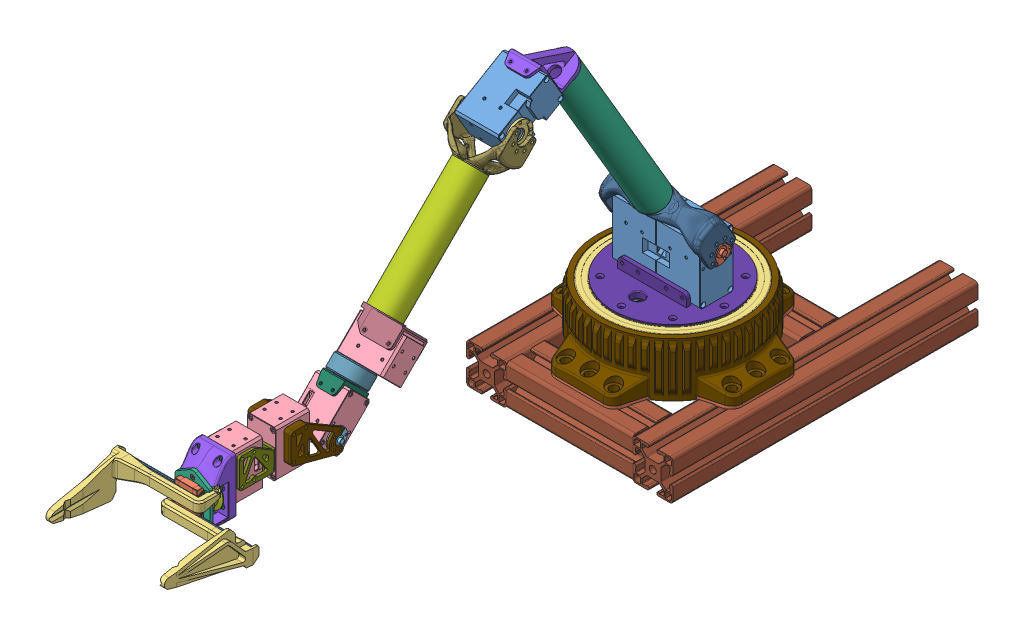
SolidWorks assembly Student_Arm, configuration Default. Lengths in mm.
Overall size (206 409.74 1579.34).
74 component instances, 44 part files, 122 mates.
Components (placement in the parent):
- Student_Arm_Geo-1: Student_Arm_Geo [Default] at origin size (0 320.38 548.3)
- Student_Arm_Geo-2: Student_Arm_Geo [Default] at (0 0 1050) x (-1 0 0) z (0 0 -1) size (0 320.38 548.3)
- XM540-1: XM540 [Default] at (22 0 0) x (0 0 -1) z (1 0 0) size (33.5 58.5 44)
- XM540-2: XM540 [Default] at (-22 0 0) x (0 0 1) z (-1 0 0) size (33.5 58.5 44)
- 540_Horn-1: 540_Horn [Default] at (22.1 0 0) x (0 0.506986 -0.861954) z (1 0 0) size (26 26 7.8)
- 540_Horn-3: 540_Horn [Default] at (-22.1 0 0) x (0 0.861954 0.506986) z (-1 0 0) size (26 26 7.8)
- XM540-3: XM540 [Default] at (0 176.7767 176.7767) x (0 -0.861954 -0.506986) z (-1 0 0) size (33.5 58.5 44)
- 540_Horn-5: 540_Horn [Default] at (0 176.7767 176.7767) x (0 0.707107 0.707107) z (-1 0 0) size (26 26 7.8)
- 540_Idler-1: 540_Idler [Default] at (0 176.7767 176.7767) x (0 -0.707107 0.707107) z (-1 0 0) size (26 26 2.5)
- 540_Dual_Frame_Custom-1: 540_Dual_Frame_Custom [Default] at (0.1 21.5489 12.6747) x (0 0.506986 -0.861954) z (1 0 0) size (30 41.17 99.35) (hidden)
- XM430-1: XM430 [Default] at (0 49.6743 303.8791) x (0 0.707107 0.707107) z (0 -0.707107 0.707107) size (28.5 46.5 34)
- XM430_Horn-1: XM430_Horn [Default] at (0 49.6743 303.8791) x (1 0 0) z (0 -0.707107 0.707107) size (19.5 19.5 6.4)
- XM430-2: XM430 [Default] at (0 0 353.5534) x (0 0.707107 0.707107) z (1 0 0) size (28.5 46.5 34)
- XM430_Horn-2: XM430_Horn [Default] at (0 0 353.5534) x (0 0.695118 -0.718895) z (1 0 0) size (19.5 19.5 6.4)
- XM430_Horn-3: XM430_Horn [Default] at (0 0 393.709) x (-0.397799 -0.917472 0) z (0 0 1) size (19.5 19.5 6.4)
- XM430-3: XM430 [Default] at (0 0 393.709) x (-1 0 0) z (0 0 1) size (28.5 46.5 34)
- L23_Tube-1: L23_Tube [Default] at origin size (30 170.86 117.41)
- L34_Tube-2: L34_Tube [Default] at origin size (30 106.83 106.83)
- J3_Mount-1: J3_Mount [Combined Plug] at origin size (30 319.78 548.3)
- XM430_Idler-1: XM430_Idler [Default] at (0 0 353.5534) x (0 0 -1) z (1 0 0) size (19.5 19.5 2)
- XM540-4: XM540 [Default] at (0 -75.35 0) x (-1 0 0) z (0 1 0) size (33.5 58.5 44)
- 540_Horn-6: 540_Horn [Default] at (0 -75.25 0) x (-0.04602 0 0.998941) z (0 1 0) size (26 26 7.8)
- L23_Mount_PostGen_V2-1: L23_Mount_PostGen_V2 [Default] at (-0.6 0 0) size (100.03 65.6 53.63)
- Base_Master-1: Base_Master [Default] at origin size (186.5 322.95 596.8) (hidden)
- 4040-1: 4040 [12in] at (-83 -119.925 -49.4) size (40 40 304.8)
- 4040-2: 4040 [12in] at (83 -119.925 -49.4) x (-1 0 0) z (0 0 -1) size (40 40 304.8)
- 4040-3: 4040 [126mm] at (-89.4 -119.925 -83) x (0 0 1) z (-1 0 0) size (40 40 126)
- 4040-4: 4040 [126mm] at (89.4 -119.925 83) x (0 0 -1) z (1 0 0) size (40 40 126)
- L34_Mount_PostGen-2: L34_Mount_PostGen [Default] at origin size (57.21 58.89 58.89)
- J4_Mount_CNC-1: J4_Mount_CNC [Default] at origin size (49.25 223.12 338.33)
- J5_Bearing_Housing-1: J5_Bearing_Housing [Default] at origin size (35 33.23 33.23)
- J5_Output-1: J5_Output [Default] at origin size (22 37.83 37.83)
- J5_Spacer-1: J5_Spacer [Default] at origin size (27 21.92 21.92)
- 4668K256_Permanently Lubricated Stainless Steel Ball Bearing-1: 4668K256_Permanently Lubricated Stainless Steel Ball Bearing [4668K256] at (0 29.1682 324.3852) x (1 0 0) z (0 -0.707107 0.707107) size (27 27 4)
- 4668K256_Permanently Lubricated Stainless Steel Ball Bearing-2: 4668K256_Permanently Lubricated Stainless Steel Ball Bearing [4668K256] at (0 34.825 318.7284) x (1 0 0) z (0 -0.707107 0.707107) size (27 27 4)
- J6_Mount-1: J6_Mount [Default] at origin size (43.08 42 52.16)
- J5_Bearing_Mount-3: J5_Bearing_Mount [Default] at origin size (54.25 320.38 548.3) (hidden)
- Gripper_Assy-1: Gripper_Assy [Default] at origin size (135.15 64.73 143.19)
  - Gripper_Geo-1: Gripper_Geo [Default] at origin size (140.5 320.38 611.55) (hidden)
  - MGN7_Rail-1: MGN7_Rail [80mm] at (24.4268 9 485.409) x (0 1 0) z (-1 0 0) size (7 4.8 80)
  - MGN7_Rail-2: MGN7_Rail [80mm] at (75.5732 -9 485.409) x (0 1 0) z (-1 0 0) size (7 4.8 80)
  - MGN7C_Carriage-1: MGN7C_Carriage [Default] at (0 9 482.959) x (0 -1 0) z (1 0 0) size (17 6.5 23.48)
  - MGN7C_Carriage-2: MGN7C_Carriage [Default] at (0 -9 482.959) x (0 -1 0) z (1 0 0) size (17 6.5 23.48)
  - Gripper_Jaw-1: Gripper_Jaw [Default] at (2.6768 0 0.1) size (88 34.92 96.64)
  - Gripper_Jaw-2: Gripper_Jaw [Default] at (-2.6768 0 0.1) x (-1 0 0) z (0 0 1) size (88 34.92 96.64)
  - XM430-1: XM430 [Default] at (0 0 440.709) x (-1 0 0) z (0 0 1) size (28.5 46.5 34)
  - XC430_Horn-1: XC430_Horn [Default] at (0 0 442.209) x (-0.461728 0.887021 0) z (0 0 1) size (20.5 20.5 5.4)
  - 9293K111_Constant-Force Spring-1: 9293K111_Constant-Force Spring [9293K111] at (0 20.4659 473.1591) x (0 0 1) z (0 -1 0) size (4.75 11.59 8.52)
  - Gripper_Carriage_Mount-1: Gripper_Carriage_Mount [Default] at origin size (34.5 52.93 3.17)
  - Gripper_Drive_Pulley-1: Gripper_Drive_Pulley [Default] at (0 0 1.5) x (0.999857 -0.016895 0) z (0 0 1) size (29.31 29.31 13.21)
  - Gripper_Structure-1: Gripper_Structure [Default] at origin size (34.93 64.73 22.83)
  - CF_Spring_Idler-1: CF_Spring_Idler [Default] at (11.3305 3.4226 0) x (0.832765 0.553627 0) z (0 0 1) size (8.62 8.62 6.75)
  - CF_Spring_Idler-2: CF_Spring_Idler [Default] at (13.8894 -35.4971 0) x (0.734452 0.678661 0) z (0 0 1) size (8.62 8.62 6.75)
  - 91292A831_18-8 Stainless Steel Socket Head Screw-1: 91292A831_18-8 Stainless Steel Socket Head Screw [91292A831] at (55.5732 -9 491.309) x (-0.599094 -0.800678 0) z (0 0 1) size (3.8 3.8 8.1)
  - 91292A835_18-8 Stainless Steel Socket Head Screw-1: 91292A835_18-8 Stainless Steel Socket Head Screw [91292A835] at (0.1352 7.9989 458.4182) x (-0.923728 -0.383049 0) z (0 0 -1) size (3.8 3.8 16.14)
  - 92125A051_18-8 Stainless Steel Hex Drive Flat Head Screw-1: 92125A051_18-8 Stainless Steel Hex Drive Flat Head Screw [92125A051] at (-4 15 479.174) x (-1 0 0) z (0 0 -1) size (4 4 5.21)
  - 92125A059_18-8 Stainless Steel Hex Drive Flat Head Screw-1: 92125A059_18-8 Stainless Steel Hex Drive Flat Head Screw [92125A059] at (0 20.4659 471.569) size (4 4 16.28)
  - 92010A775_Passivated 18-8 Stainless Steel Phillips Flat Head Screw-1: 92010A775_Passivated 18-8 Stainless Steel Phillips Flat Head Screw [92010A775] at (-11 8 459.309) size (4.7 4.7 6.14)
  - 92125A085_18-8 Stainless Steel Hex Drive Flat Head Screw-1: 92125A085_18-8 Stainless Steel Hex Drive Flat Head Screw [92125A085] at (-11 32 461.139) size (5 5 16.3)
  - 92125A085_18-8 Stainless Steel Hex Drive Flat Head Screw-2: 92125A085_18-8 Stainless Steel Hex Drive Flat Head Screw [92125A085] at (11 32 461.139) x (0.987351 0.158553 0) z (0 0 1) size (5 5 16.3)
  - 92125A085_18-8 Stainless Steel Hex Drive Flat Head Screw-4: 92125A085_18-8 Stainless Steel Hex Drive Flat Head Screw [92125A085] at (11 -8 461.139) x (0.959125 0.282984 0) z (0 0 1) size (5 5 16.3)
  - 92125A085_18-8 Stainless Steel Hex Drive Flat Head Screw-6: 92125A085_18-8 Stainless Steel Hex Drive Flat Head Screw [92125A085] at (-11 -8 461.139) x (0.928571 0.371154 0) z (0 0 1) size (5 5 16.3)
  - 92010A775_Passivated 18-8 Stainless Steel Phillips Flat Head Screw-2: 92010A775_Passivated 18-8 Stainless Steel Phillips Flat Head Screw [92010A775] at (11 8 459.309) x (0.987351 0.158553 0) z (0 0 1) size (4.7 4.7 6.14)
  - 92125A059_18-8 Stainless Steel Hex Drive Flat Head Screw-2: 92125A059_18-8 Stainless Steel Hex Drive Flat Head Screw [92125A059] at (0 -20.4659 471.569) x (0.987351 0.158553 0) z (0 0 1) size (4 4 16.28)
  - 91292A835_18-8 Stainless Steel Socket Head Screw-2: 91292A835_18-8 Stainless Steel Socket Head Screw [91292A835] at (7.9989 -0.1352 458.4182) x (-0.85131 -0.524663 0) z (0 0 -1) size (3.8 3.8 16.14)
  - 91292A835_18-8 Stainless Steel Socket Head Screw-3: 91292A835_18-8 Stainless Steel Socket Head Screw [91292A835] at (-0.1352 -7.9989 458.4182) x (-0.777574 -0.628792 0) z (0 0 -1) size (3.8 3.8 16.14)
  - 91292A835_18-8 Stainless Steel Socket Head Screw-4: 91292A835_18-8 Stainless Steel Socket Head Screw [91292A835] at (-7.9989 0.1352 458.4182) x (-0.715577 -0.698533 0) z (0 0 -1) size (3.8 3.8 16.14)
- G_Mount-1: G_Mount [Default] at origin size (33.58 46.5 37)
- J1_Top_Plate-1: J1_Top_Plate [Default] at (0 -0.6 0) size (119 28.25 119)
- J1_Enclosure-1: J1_Enclosure [Default] at (0 -0.6 0) size (186.5 53.92 186.5)
- J1_Inner_Joint-1: J1_Inner_Joint [Default] x (0.993975 0 0.109606) z (-0.109606 0 0.993975) size (119 33.75 119)
- J1_Mount-1: J1_Mount [Default] at (0 -0.6 0) size (186 3.17 186)
- 6822-2Z-1: 6822-2Z [Default] at (0 -76.75 0) x (0.938147 0 -0.346237) z (0.346237 0 0.938147) size (140 16.01 140)
- 6822-2Z-2: 6822-2Z [Default] at (0 -46.6 0) x (0.938147 0 -0.346237) z (0.346237 0 0.938147) size (140 16.01 140)
Mates (geometry in assembly coordinates):
- Coincident1: coincident anti-aligned: plane of XM540-1 through (0 12.3693 4) normal (-1 0 0); plane of XM540-2 through (0 12.3693 -4) normal (1 0 0)
- Coincident2: coincident aligned: plane of XM540-1 through (0 -44.75 -16.75) normal (0 0 -1); plane of XM540-2 through (0 13.75 -16.75) normal (0 0 -1)
- Coincident3: coincident aligned: plane of XM540-1 through (0 13.75 -16.75) normal (0 1 0); plane of XM540-2 through (0 13.75 16.75) normal (0 1 0)
- Coincident4: coincident anti-aligned: plane of XM540-1 through (0 12.3693 4) normal (-1 0 0)
- Coincident5: coincident: line of XM540-1 through (0 59.73 54.515) axis (0 0 -1)
- Parallel1: parallel aligned: plane of XM540-1 through (22 0 0) normal (0 1 0)
- Concentric1: concentric aligned: line of XM540-1 through (0 59.73 54.515) axis (0 0 -1); cylinder of 540_Horn-1 through (49.35 0 0) axis (-1 0 0) radius 13
- Concentric2: concentric aligned: line of XM540-2 through (0 59.73 -54.515) axis (0 0 1); cylinder of 540_Horn-3 through (-49.35 0 0) axis (1 0 0) radius 13
- Concentric3: concentric aligned: line of XM540-3 through (-32.515 176.7767 176.7767) axis (1 0 0); cylinder of 540_Horn-5 through (-27.25 176.7767 176.7767) axis (1 0 0) radius 13
- Coincident8: coincident anti-aligned: plane of XM540-3 through (-22 157.4374 180.8897) normal (-1 0 0); plane of 540_Horn-5 through (-22 196.5292 177.6495) normal (1 0 0)
- Concentric4: concentric aligned: line of XM540-3 through (-32.515 176.7767 176.7767) axis (1 0 0); cylinder of 540_Idler-1 through (21.875 176.7767 176.7767) axis (1 0 0) radius 13
- Coincident9: coincident anti-aligned: plane of XM540-3 through (22 173.9534 189.4664) normal (1 0 0); plane of 540_Idler-1 through (22 188.3516 182.6947) normal (-1 0 0)
- Coincident10: coincident anti-aligned: plane of 540_Horn-1 through (46.6 0 0) normal (1 0 0); plane of 540_Dual_Frame_Custom-1 through (46.6 21.5489 12.6747) normal (-1 0 0)
- Concentric5: concentric anti-aligned: cylinder of 540_Horn-1 through (49.35 0 0) axis (-1 0 0) radius 5; cylinder of 540_Dual_Frame_Custom-1 through (-49.575 0 0) axis (1 0 0) radius 5.25
- Concentric6: concentric aligned: cylinder of 540_Horn-1 through (43.3283 9.4815 5.5769) axis (1 0 0) radius 1.025; cylinder of 540_Dual_Frame_Custom-1 through (-49.575 9.4815 5.5769) axis (1 0 0) radius 1.35
- Concentric7: concentric anti-aligned: cylinder of 540_Horn-3 through (-43.3283 9.4815 5.5769) axis (-1 0 0) radius 1.025; cylinder of 540_Dual_Frame_Custom-1 through (-49.575 9.4815 5.5769) axis (1 0 0) radius 1.35
- Coincident11: coordinate: unknown of Student_Arm_Geo-1
- Coincident12: coincident: unknown of ?; line of XM540-3 through (-32.515 176.7767 176.7767) axis (1 0 0)
- Coincident16: coincident: line of Student_Arm_Geo-1 through (0 184.2434 197.1206) axis (0 0.506986 -0.861954); plane of XM540-3 through (22 184.2434 197.1206) normal (0 0.861954 0.506986)
- Width3: width anti-aligned: plane of XM540-3 through (-22 157.4374 180.8897) normal (-1 0 0); plane of XM540-1 through (22 176.7767 176.7767) normal (1 0 0); plane of XM540-3 through (44 13.35 -14.5843) normal (1 0 0); plane of XM540-2 through (-44 13.35 14.5843) normal (-1 0 0)
- Coincident17: coincident anti-aligned: plane of 540_Horn-5 through (-24.5 176.7767 176.7767) normal (-1 0 0); plane of FR13_H101-1 through (-24.5 177.8374 156.6242) normal (1 0 0)
- Concentric8: concentric aligned: cylinder of 540_Horn-5 through (-27.25 176.7767 176.7767) axis (1 0 0) radius 5; cylinder of FR13_H101-1 through (-25.5 176.7767 176.7767) axis (1 0 0) radius 5
- Concentric10: concentric aligned: cylinder of 540_Horn-5 through (-21.2283 184.5549 184.5549) axis (-1 0 0) radius 1.025; cylinder of FR13_H101-1 through (26.5 184.5549 184.5549) axis (-1 0 0) radius 1.25
- Concentric11: concentric anti-aligned: cylinder of 540_Idler-1 through (21.2283 184.5549 184.5549) axis (1 0 0) radius 1.025; cylinder of FR13_H101-1 through (26.5 184.5549 184.5549) axis (-1 0 0) radius 1.25
- Parallel3: parallel aligned: plane of FR13_H101-1 through (12.3328 166.8772 209.3036) normal (0 0.707107 0.707107); plane of XM430-1 through (35.25 71.7713 301.9346) normal (0 0.707107 0.707107)
- Coincident20: coincident anti-aligned: plane of XM430-1 through (-10.85 46.1983 324.4449) normal (0 -0.707107 0.707107); plane of XM430_Horn-1 through (12.0843 45.3255 323.5721) normal (0 0.707107 -0.707107)
- Concentric12: concentric anti-aligned: line of XM430-1 through (0 62.8981 290.6553) axis (0 -0.707107 0.707107); cylinder of XM430_Horn-1 through (0 34.5775 318.9759) axis (0 0.707107 -0.707107) radius 9.75
- Coincident21: coincident aligned: line of Student_Arm_Geo-1 through (0 176.7767 176.7767) axis (0 -0.707107 0.707107); line of XM430-1 through (0 62.8981 290.6553) axis (0 -0.707107 0.707107)
- Coincident22: coincident: line of Student_Arm_Geo-1 through (0 47.7297 325.9762) axis (0 -0.707107 -0.707107); plane of XM430-1 through (-10.85 46.1983 324.4449) normal (0 -0.707107 0.707107)
- Concentric13: concentric anti-aligned: line of XM430-2 through (-18.7013 0 353.5534) axis (1 0 0); cylinder of XM430_Horn-2 through (21.35 0 353.5534) axis (-1 0 0) radius 9.75
- Coincident23: coincident anti-aligned: plane of XM430-2 through (17 0.8728 369.7704) normal (1 0 0); plane of XM430_Horn-2 through (17 16.2 352.4081) normal (-1 0 0)
- Coincident25: coincident: unknown of ?; line of XM430-2 through (-18.7013 0 353.5534) axis (1 0 0)
- Width4: width aligned: plane of XM430-2 through (17 0.8728 369.7704) normal (1 0 0); plane of XM540-1 through (-17 0 353.5534) normal (-1 0 0); plane of XM430-2 through (44 13.35 -14.5843) normal (1 0 0); plane of XM540-2 through (-44 13.35 14.5843) normal (-1 0 0)
- Coincident26: coincident: line of Student_Arm_Geo-1 through (0 2.1213 371.5846) axis (0 0.707107 -0.707107); plane of XM430-2 through (-17 35.0018 338.7041) normal (0 0.707107 0.707107)
- Coincident27: coincident anti-aligned: line of Student_Arm_Geo-1 through (0 0 353.5534) axis (0 0 1); line of XC430-1 through (0 0 459.4285) axis (0 0 -1)
- Concentric14: concentric anti-aligned: cylinder of XM430_Horn-3 through (0 0 415.059) axis (0 0 -1) radius 9.75; line of XM430-3 through (0 0 375.0076) axis (0 0 1)
- Coincident31: coincident anti-aligned: plane of XM430_Horn-3 through (5.1474 -15.4031 410.709) normal (0 0 -1); plane of XM430-3 through (-12.0843 -10.85 410.709) normal (0 0 1)
- Coincident32: coincident aligned: line of Student_Arm_Geo-1 through (0 0 353.5534) axis (0 0 1); line of XM430-3 through (0 0 375.0076) axis (0 0 1)
- Concentric16: concentric anti-aligned: cylinder of L23_Tube-1 through (0 0 0) axis (0 -0.861954 -0.506986) radius 13; cylinder of Glue_In_Plug-2 through (0 224.037 131.7747) axis (0 0.861954 0.506986) radius 12.95
- Concentric17: concentric aligned: cylinder of L34_Tube-2 through (0 176.7767 176.7767) axis (0 0.707107 -0.707107) radius 13; cylinder of Glue_In_Plug-4 through (0 179.6051 173.9483) axis (0 0.707107 -0.707107) radius 12.95
- Coincident37: coincident anti-aligned: plane of L34_Tube-2 through (0 -25.2231 25.2231) normal (0 0.707107 -0.707107); plane of Glue_In_Plug-4 through (-6.6363 161.0657 211.5119) normal (0 -0.707107 0.707107)
- Concentric18: concentric anti-aligned: cylinder of L34_Tube-2 through (0 176.7767 176.7767) axis (0 0.707107 -0.707107) radius 13; cylinder of Glue_In_Plug-6 through (0 37.8862 315.6672) axis (0 -0.707107 0.707107) radius 12.95
- Coincident39: coincident anti-aligned: plane of L23_Tube-1 through (0 189.8426 111.6621) normal (0 0.861954 0.506986); plane of Glue_In_Plug-2 through (-7.8715 183.369 122.6682) normal (0 -0.861954 -0.506986)
- Concentric19: concentric anti-aligned: cylinder of XC430-1 through (0 0 425.599) axis (0 0 -1) radius 10.5; cylinder of XC430_Idler-1 through (0 0 421.534) axis (0 0 1) radius 10.25
- Distance1: distance = 2 mm aligned: plane of XC430_Idler-1 through (0 0 421.709) normal (0 0 -1); plane of XC430-1 through (0 0 423.709) normal (0 0 -1)
- Distance2: distance = 2 mm aligned: plane of XC430-1 through (0 0 457.709) normal (0 0 1); plane of XC430_Horn-1 through (0 0 459.709) normal (0 0 1)
- Concentric21: concentric aligned: cylinder of XC430-1 through (0 0 457.709) axis (0 0 1) radius 10.4; cylinder of XC430_Horn-1 through (0 0 456.209) axis (0 0 1) radius 10.25
- Concentric22: concentric anti-aligned: line of XM430-2 through (-18.7013 0 353.5534) axis (1 0 0); cylinder of XM430_Idler-1 through (-16 0 353.5534) axis (-1 0 0) radius 9.75
- Coincident41: coincident anti-aligned: plane of XM430-2 through (-17 -5.1972 363.7004) normal (-1 0 0); plane of XM430_Idler-1 through (-17 10.85 350.0534) normal (1 0 0)
- Concentric23: concentric anti-aligned: line of XM540-4 through (0 -42.835 0) axis (0 -1 0); cylinder of 540_Horn-6 through (0 -48.45 0) axis (0 1 0) radius 2.75
- Coincident43: coincident aligned: line of Student_Arm_Geo-1 through (44 0 -53.35) axis (0 0 -1); line of XM540-4 through (0 -42.835 0) axis (0 -1 0)
- Coincident44: coincident: line of Student_Arm_Geo-1 through (0 -53.35 -44.75) axis (0 -1 0); plane of XM540-4 through (16.75 -97.35 -44.75) normal (0 0 -1)
- Coincident45: coincident: line of Student_Arm_Geo-1 through (0 -97.35 13.75) axis (0 0 -1); plane of XM540-4 through (0 -97.35 0) normal (0 -1 0)
- Coincident46: coincident anti-aligned: plane of L34_Tube-2 through (0 -110.839 110.839) normal (0 -0.707107 0.707107); plane of Glue_In_Plug-6 through (2.4176 55.4698 277.1477) normal (0 0.707107 -0.707107)
- Coincident47: coincident anti-aligned: plane of 540_Horn-3 through (-46.6 0 0) normal (-1 0 0); plane of L23_Mount_PostGen_V2-1 through (-46.6 0 0) normal (1 0 0)
- Concentric24: concentric aligned: cylinder of 540_Horn-3 through (-49.35 0 0) axis (1 0 0) radius 5; cylinder of L23_Mount_PostGen_V2-1 through (-50.6 0 0) axis (1 0 0) radius 7
- Concentric25: concentric anti-aligned: cylinder of 540_Horn-3 through (-43.3283 5.5769 -9.4815) axis (-1 0 0) radius 1.025; cylinder of L23_Mount_PostGen_V2-1 through (-50.6 5.5769 -9.4815) axis (1 0 0) radius 1.35
- Concentric27: concentric anti-aligned: cylinder of Base_Master-1 through (0 -112.0875 0) axis (0 -1 0) radius 70; cylinder of 6822-2Z-1 through (0 -84.75 0) axis (0 1 0) radius 70
- Coincident50: coincident anti-aligned: plane of Base_Master-1 through (66 -76.75 0) normal (0 -1 0); plane of 6822-2Z-1 through (23.1546 -76.75 62.7386) normal (0 1 0)
- Coincident52: coincident: line of Student_Arm_Geo-1 through (0 -50.75 13) axis (0 0 -1); plane of 540_Horn-6 through (0 -50.75 0) normal (0 1 0)
- Coincident53: coincident: plane of 540_Horn-3 through (-46.6 0 0) normal (-1 0 0); line of Base_Master-1 through (26 -46.6 -13) axis (0 0 1)
- Coincident54: coincident: plane of 540_Horn-1 through (46.6 0 0) normal (1 0 0); line of Base_Master-1 through (26 46.6 13) axis (0 0 -1)
- Parallel6: parallel aligned: cylinder of L23_Tube-1 through (0 0 0) axis (0 -0.861954 -0.506986) radius 13; cylinder of L23_Mount_PostGen_V2-1 through (-0.6 0 0) axis (0 -0.861954 -0.506986) radius 12.95
- Coincident55: coincident anti-aligned: plane of Base_Master-1 through (0 -99.925 0) normal (0 -1 0); plane of 4040-1ft-1 through (-66 -99.925 103) normal (0 1 0)
- Distance3: distance = 20 mm: cylinder of Base_Master-1 through (-83 -99.925 0) axis (0 1 0) radius 4.25; plane of 4040-1ft-1 through (-103 -102.925 103) normal (-1 0 0)
- Parallel7: parallel aligned: plane of Base_Master-1 through (-93 -362.9687 -24) normal (-1 0 0); plane of 4040-1ft-1 through (-103 -102.925 103) normal (-1 0 0)
- Coincident57: coincident anti-aligned: plane of Base_Master-1 through (0 -99.925 0) normal (0 -1 0); plane of 4040-1ft-2 through (66 -99.925 -201.8) normal (0 1 0)
- Distance4: distance = 20 mm: cylinder of Base_Master-1 through (83 -96.75 0) axis (0 1 0) radius 4.25; plane of 4040-1ft-2 through (103 -102.925 -201.8) normal (1 0 0)
- Parallel8: parallel aligned: plane of Base_Master-1 through (93 -80.75 24) normal (1 0 0); plane of 4040-1ft-2 through (103 -102.925 -201.8) normal (1 0 0)
- Coincident58: coincident anti-aligned: plane of Base_Master-1 through (0 -99.925 0) normal (0 -1 0); plane of 4040-1ft-3 through (-241.8 -99.925 -66) normal (0 1 0)
- Distance6: distance = 20 mm: cylinder of Base_Master-1 through (0 -96.75 -83) axis (0 1 0) radius 4.25; plane of 4040-1ft-3 through (-241.8 -102.925 -103) normal (0 0 -1)
- Parallel9: parallel aligned: plane of Base_Master-1 through (24 -80.75 -93) normal (0 0 -1); plane of 4040-1ft-3 through (-241.8 -102.925 -103) normal (0 0 -1)
- Coincident59: coincident anti-aligned: plane of Base_Master-1 through (0 -99.925 0) normal (0 -1 0); plane of 4040-1ft-4 through (241.8 -99.925 66) normal (0 1 0)
- Distance7: distance = 20 mm: cylinder of Base_Master-1 through (0 -96.75 83) axis (0 1 0) radius 4.25; plane of 4040-1ft-4 through (241.8 -102.925 103) normal (0 0 1)
- Parallel10: parallel aligned: plane of Base_Master-1 through (-24 -80.75 93) normal (0 0 1); plane of 4040-1ft-4 through (241.8 -102.925 103) normal (0 0 1)
- Coincident61: coincident anti-aligned: plane of Student_Arm_Geo-2 through (0 0 1050) normal (-1 0 0)
- Coincident62: coincident aligned: plane of Student_Arm_Geo-1 through (0 0 0) normal (0 1 0); plane of Student_Arm_Geo-2 through (0 0 1050) normal (0 1 0)
- Distance8: distance = 1050 mm: line of Student_Arm_Geo-1 through (44 0 -53.35) axis (0 0 -1); line of Student_Arm_Geo-2 through (0 -53.35 1050) axis (0 -1 0)
- Concentric29: concentric anti-aligned: cylinder of 540_Idler-1 through (21.875 176.7767 176.7767) axis (1 0 0) radius 5; cylinder of L34_Mount_PostGen-1 through (28.5 176.7767 176.7767) axis (-1 0 0) radius 7
- Coincident63: coincident anti-aligned: plane of 540_Idler-1 through (24.5 176.7767 176.7767) normal (1 0 0); plane of L34_Mount_PostGen-1 through (24.5 353.5534 353.5534) normal (-1 0 0)
- Parallel11: parallel aligned: cylinder of L34_Tube-2 through (0 176.7767 176.7767) axis (0 0.707107 -0.707107) radius 13; cylinder of L34_Mount_PostGen-1 through (-0.1 179.6051 173.9483) axis (0 0.707107 -0.707107) radius 12.95
- Coincident64: coincident anti-aligned: plane of 4040-2 through (63 -102.925 -201.8) normal (-1 0 0); plane of 4040-4 through (63 -136.925 66) normal (1 0 0)
- Coincident65: coincident anti-aligned: plane of 4040-1 through (-63 -102.925 103) normal (1 0 0); plane of 4040-3 through (-63 -136.925 -66) normal (-1 0 0)
- Coincident66: coincident aligned: plane of 4040-1 through (-66 -136.925 103) normal (0 0 1); plane of 4040-4 through (241.8 -102.925 103) normal (0 0 1)
- Coincident67: coincident aligned: plane of 4040-2 through (66 -136.925 103) normal (0 0 1); plane of 4040-4 through (241.8 -102.925 103) normal (0 0 1)
- Concentric30: concentric anti-aligned: cylinder of L34_Tube-2 through (0 176.7767 176.7767) axis (0 0.707107 -0.707107) radius 13; cylinder of J4_Mount_CNC-1 through (0 37.8862 315.6672) axis (0 -0.707107 0.707107) radius 10.95
- Coincident68: coincident anti-aligned: plane of L34_Tube-2 through (0 -110.839 110.839) normal (0 -0.707107 0.707107); plane of J4_Mount_CNC-1 through (0 55.3311 277.0091) normal (0 0.707107 -0.707107)
- Coincident69: coincident aligned: plane of J4_Mount_CNC-1 through (0 0 0) normal (1 0 0)
- Coincident70: coincident: line of Student_Arm_Geo-1 through (0 -11.25 410.709) axis (0 1 0); plane of XM430-3 through (-12.0843 -10.85 410.709) normal (0 0 1)
- Coincident72: coincident: line of Student_Arm_Geo-1 through (0 14.25 457.709) axis (0 -1 0); plane of XC430-1 through (0 0 457.709) normal (0 0 1)
- Concentric33: concentric anti-aligned: cylinder of J4_Bearing_Housing-1 through (0 1.2392 352.3142) axis (0 0.707107 -0.707107) radius 10.5; cylinder of 4668K256_Permanently Lubricated Stainless Steel Ball Bearing-2 through (0 33.4108 320.1426) axis (0 -0.707107 0.707107) radius 13.5
- Coincident74: coincident anti-aligned: plane of J4_Bearing_Housing-1 through (0 -140.5375 140.5375) normal (0 -0.707107 0.707107); plane of 4668K256_Permanently Lubricated Stainless Steel Ball Bearing-2 through (0 45.7035 326.7785) normal (0 0.707107 -0.707107)
- Concentric34: concentric aligned: cylinder of J4_Bearing_Housing-1 through (0 1.2392 352.3142) axis (0 0.707107 -0.707107) radius 10.5; cylinder of J4_Spacer-1 through (0 176.7767 176.7767) axis (0 0.707107 -0.707107) radius 12.5
- Coincident75: coincident anti-aligned: plane of J4_Spacer-1 through (0 -143.3659 143.3659) normal (0 0.707107 -0.707107); plane of 4668K256_Permanently Lubricated Stainless Steel Ball Bearing-2 through (0 42.8751 329.6069) normal (0 -0.707107 0.707107)
- Concentric35: concentric anti-aligned: cylinder of J4_Bearing_Housing-1 through (0 1.2392 352.3142) axis (0 0.707107 -0.707107) radius 10.5; cylinder of 4668K256_Permanently Lubricated Stainless Steel Ball Bearing-1 through (0 27.7539 325.7994) axis (0 -0.707107 0.707107) radius 13.5
- Coincident76: coincident anti-aligned: plane of J4_Spacer-1 through (0 -146.1943 146.1943) normal (0 -0.707107 0.707107); plane of 4668K256_Permanently Lubricated Stainless Steel Ball Bearing-1 through (0 40.0467 332.4353) normal (0 0.707107 -0.707107)
- Concentric36: concentric aligned: cylinder of J4_Bearing_Housing-1 through (0 1.2392 352.3142) axis (0 0.707107 -0.707107) radius 10.5; cylinder of J4_Output-1 through (0 176.7767 176.7767) axis (0 0.707107 -0.707107) radius 10
- Coincident77: coincident anti-aligned: plane of J4_Output-1 through (0 -149.0228 149.0228) normal (0 0.707107 -0.707107); plane of 4668K256_Permanently Lubricated Stainless Steel Ball Bearing-1 through (0 34.9594 333.0049) normal (0 -0.707107 0.707107)
- Concentric37: concentric aligned: cylinder of XM430_Horn-1 through (0 34.5775 318.9759) axis (0 0.707107 -0.707107) radius 9.75; cylinder of J4_Bearing_Housing-1 through (0 1.2392 352.3142) axis (0 0.707107 -0.707107) radius 10.5
- Concentric38: concentric aligned: cylinder of XM430-1 through (8 48.4875 320.6222) axis (0 -0.707107 0.707107) radius 1.025; cylinder of J4_Bearing_Housing-1 through (8 44.0174 325.0923) axis (0 -0.707107 0.707107) radius 1.35
- Coincident78: coincident anti-aligned: plane of XM430-1 through (-10.85 46.1983 324.4449) normal (0 -0.707107 0.707107); plane of J4_Bearing_Housing-1 through (0 -139.1233 139.1233) normal (0 0.707107 -0.707107)
- Coincident79: coincident: line of Student_Arm_Geo-1 through (0 35.25 376.709) axis (0 0 1); plane of XM430-3 through (14.25 35.25 376.709) normal (0 1 0)
- Coincident83: coincident anti-aligned: plane of XC430_Horn-1 through (0 0 461.609) normal (0 0 1); plane of MGN7_Rail-1 through (10.581 3.4794 461.609) normal (0 0 -1)
- Parallel12: parallel anti-aligned: plane of MGN7_Rail-1 through (10.581 3.2794 461.809) normal (0 -1 0)
- Coincident85: coincident aligned: plane of Gripper_Assy-1 through (0 0 0) normal (1 0 0)
- Coincident86: coincident: line of Student_Arm_Geo-1 through (0 -11.25 457.709) axis (0 1 0); plane of Gripper_Assy-1/XM430-1 through (-12.0843 -10.85 457.709) normal (0 0 1)
- Coincident87: coincident aligned: line of Student_Arm_Geo-1 through (0 0 353.5534) axis (0 0 1); line of Gripper_Assy-1/XM430-1 through (0 0 422.0076) axis (0 0 1)
- Concentric39: concentric aligned: cylinder of XM430_Horn-3 through (0 0 415.059) axis (0 0 -1) radius 4; cylinder of G_Mount-1 through (0 0 415.249) axis (0 0 -1) radius 5
- Concentric40: concentric aligned: cylinder of Gripper_Assy-1/XM430-1 through (-10.4533 4 446.709) axis (-1 0 0) radius 1.025; cylinder of G_Mount-1 through (-16.79 4 446.709) axis (-1 0 0) radius 1.45
- Coincident88: coincident anti-aligned: plane of XM540-4 through (4 -97.35 12.3693) normal (0 -1 0); plane of J1_Mount-1 through (-24 -97.35 83) normal (0 1 0)
- Concentric41: concentric aligned: cylinder of XM540-4 through (13.5 -97.35 10.5) axis (0 -1 0) radius 2.4; cylinder of J1_Mount-1 through (13.5 -100.525 10.5) axis (0 -1 0) radius 1.45
- Concentric42: concentric aligned: cylinder of XM540-4 through (-13.5 -97.35 10.5) axis (0 -1 0) radius 2.4; cylinder of J1_Mount-1 through (-13.5 -100.525 10.5) axis (0 -1 0) radius 1.45
- Coincident89: coincident anti-aligned: plane of J1_Enclosure-1 through (-83 -97.35 -24) normal (0 -1 0); plane of J1_Mount-1 through (-24 -97.35 83) normal (0 1 0)
- Concentric43: concentric aligned: cylinder of J1_Enclosure-1 through (-24 -97.35 83) axis (0 1 0) radius 4.25; cylinder of J1_Mount-1 through (-24 -100.525 83) axis (0 1 0) radius 4.25
- Concentric44: concentric aligned: cylinder of J1_Enclosure-1 through (24 -97.35 83) axis (0 1 0) radius 4.25; cylinder of J1_Mount-1 through (24 -100.525 83) axis (0 1 0) radius 4.25
- Concentric46: concentric anti-aligned: cylinder of J1_Enclosure-1 through (0 -112.6875 0) axis (0 -1 0) radius 70; cylinder of 6822-2Z-2 through (0 -54.6 0) axis (0 1 0) radius 70
- Coincident90: coincident anti-aligned: plane of J1_Enclosure-1 through (70 -62.6 0) normal (0 1 0); plane of 6822-2Z-2 through (23.1546 -62.6 62.7386) normal (0 -1 0)
- Concentric47: concentric aligned: cylinder of J1_Top_Plate-1 through (0 -45.35 0) axis (0 1 0) radius 55; cylinder of 6822-2Z-2 through (0 -54.6 0) axis (0 1 0) radius 55
- Coincident91: coincident anti-aligned: plane of J1_Top_Plate-1 through (-55 -46.6 0) normal (0 -1 0); plane of 6822-2Z-2 through (20.125 -46.6 54.5298) normal (0 1 0)
- Coincident92: coincident anti-aligned: plane of XM540-1 through (0 13.75 16.75) normal (0 0 1); plane of J1_Top_Plate-1 through (-30 -38.6 16.75) normal (0 0 -1)
- Concentric48: concentric anti-aligned: cylinder of J1_Inner_Joint-1 through (0 -112.0875 0) axis (0 -1 0) radius 47.7821; cylinder of 6822-2Z-1 through (0 -84.75 0) axis (0 1 0) radius 55
- Coincident93: coincident anti-aligned: plane of J1_Inner_Joint-1 through (-59.1415 -92.75 -6.5215) normal (0 1 0); plane of 6822-2Z-1 through (20.125 -92.75 54.5298) normal (0 -1 0)
